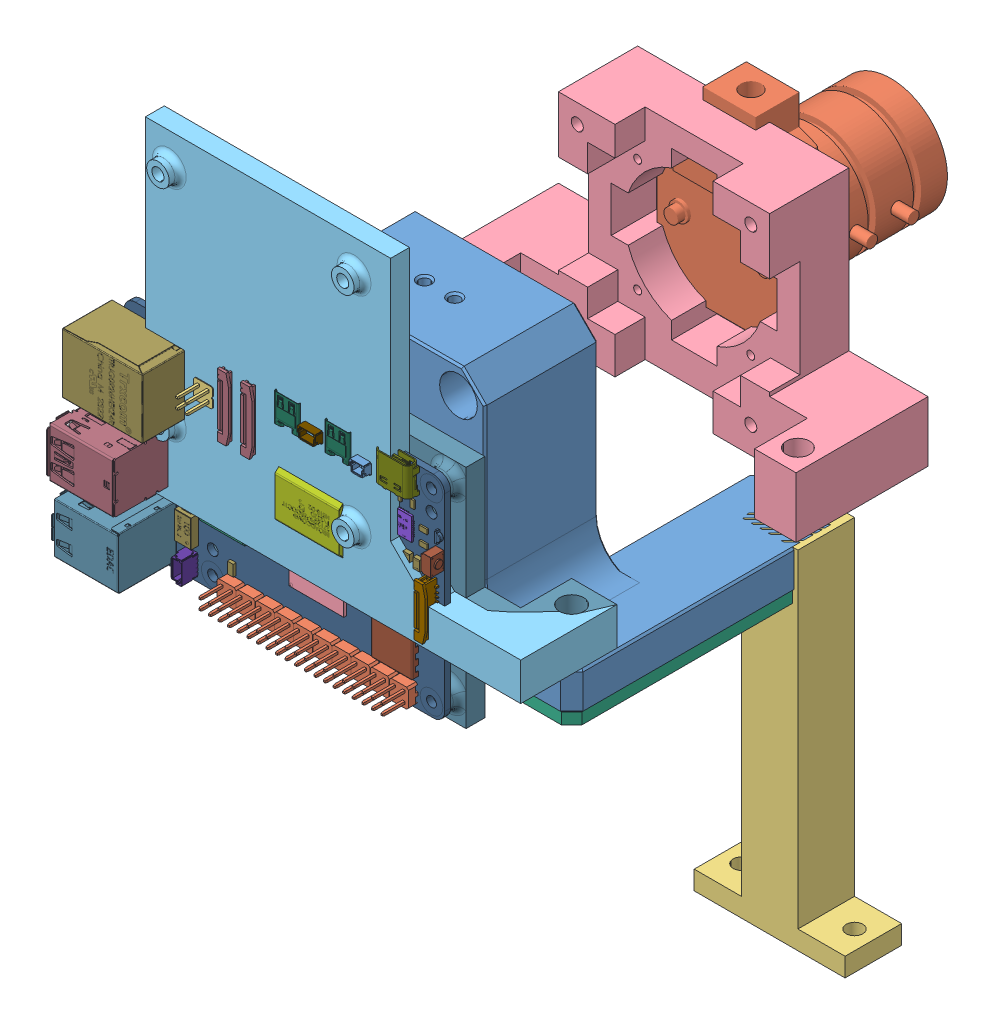
SolidWorks assembly Cam Existing setup, configuration Default. Lengths in mm.
Overall size (125.35 177 162.46).
37 component instances, 32 part files, 41 mates.
Components (placement in the parent):
- zaxismounting-1: zaxismounting [Default] at (-53.5245 -37.6157 41.3258) size (100 66.5 73)
- raspi_HQ_cam_and_6mm_lens-1: raspi_HQ_cam_and_6mm_lens [Default] at (-22.5245 33.3843 -47.4742) x (1 0 0) z (0 0 -1) size (38.99 51.7 46.02)
- Cam-Plate Spacer-1: Cam-Plate Spacer [Default] at (-3.5245 -27.6157 -51.1742) x (1 0 0) z (0 -1 0) size (40 15 92)
- Rpi Cam Mount 2-1: Rpi Cam Mount 2 [Default] at (-3.5245 2.3843 -41.1742) x (-1 0 0) z (0 0 -1) size (98 58 35)
- Rpi Mount-1: Rpi Mount [Default] at (-53.5245 -27.6157 41.3258) x (1 0 0) z (0 1 0) size (99.5 28.5 85)
- Spacer 3mm Zaxis mount^Cam Existing setup-1: Spacer 3mm Zaxis mount^Cam Existing setup [Default] at (-53.5245 -37.6157 41.3258) x (-1 0 0) z (0 -1 0) size (99 72 3)
- RASPBERRY_PI_5-2: RASPBERRY_PI_5 [Default] at (-18.9805 -16.8057 50.4258) x (-1 0 0) z (0 1 0) size (89.04 20.84 57.19)
  - RASPBERRY_PI_5.STEP-1: RASPBERRY_PI_5.STEP [Default] at origin size (89.04 20.84 57.19)
    - SLOT_CARD_ASM.STEP-1: SLOT_CARD_ASM.STEP [Default] at (-44.5448 -12.71 -6.4393) x (0 0 -1) z (0 1 0) size (11.95 11.4 1.48)
      - CARD_SLOT_METAL_PIN.STEP-1: CARD_SLOT_METAL_PIN.STEP [Default] at (-3.5293 -7.6678 12.2938) x (0 -1 0) z (1 0 0) size (7.95 0.89 8.04)
      - SD_CARD_V1.STEP-1: SD_CARD_V1.STEP [Default] at (-18.1743 -9.7848 12.71) x (-1 0 0) z (0 0 -1) size (11.71 10.28 1.3)
      - PART3_V1.STEP-1: PART3_V1.STEP [Default] at (-6.4643 -9.3448 11.38) x (1 0 0) z (0 0 -1) size (11.95 11.4 1.45)
    - PLATE_RASPBERRY_PI_5.STEP-1: PLATE_RASPBERRY_PI_5.STEP [Default] x (1 0 0) z (0 1 0) size (85 56 1.7)
    - METAL_PLATE..STEP-1: METAL_PLATE..STEP [Default] at (-30 3 -14.2) x (1 0 0) z (0 1 0) size (11.01 13.01 1.6)
    - GIGABIT_ETHERNET_PORT.STEP-1: GIGABIT_ETHERNET_PORT.STEP [Default] at (45.5 8.525 17.8) x (0 0 -1) z (1 0 0) size (16.1 17.2 21.45)
    - 2xUSB_3.0_PORT.STEP-1: 2xUSB_3.0_PORT.STEP [Default] at (28.53 10.58 -1.1) x (0 1 0) z (1 0 0) size (20.65 15.33 17.66)
    - 2xUSB_2.0_PORT.STEP-1: 2xUSB_2.0_PORT.STEP [Default] at (28.53 9.4 -19) x (0 1 0) z (1 0 0) size (19.16 15.33 17.86)
    - FEMALE_MICRO_HDMI_CONNECTOR.STEP-1: FEMALE_MICRO_HDMI_CONNECTOR.STEP [Default] at (-16.7 3.05 21.5) size (6.5 3.51 7.5)
    - FEMALE_MICRO_HDMI_CONNECTOR.STEP-2: FEMALE_MICRO_HDMI_CONNECTOR.STEP [Default] at (-3.3 3.05 21.5) size (6.5 3.51 7.5)
    - FEMALE_USB_CONNECTOR.STEP-1: FEMALE_USB_CONNECTOR.STEP [Default] at (-31.3 3.18 21.58) size (8.94 3.96 7.9)
    - STOCK_1.STEP-1: STOCK_1.STEP [Default] at (0.2694 -0.16 -24.2409) x (1 0 0) z (0 1 0) size (3.61 6 4.35)
    - STOCK_2.STEP-1: STOCK_2.STEP [Default] at (-10.7909 -0.16 48.1306) x (0 0 -1) z (0 1 0) size (3.61 5 4.35)
    - STOCK_3.STEP-1: STOCK_3.STEP [Default] at (-24.6409 -0.16 47.3806) x (0 0 -1) z (0 1 0) size (3.61 4 4.35)
    - 3.0_PIN_HEADER_10.STEP-1: 3.0_PIN_HEADER_10.STEP [Default] at (-32.86 4.1 -24.5) x (0 0 -1) z (0 1 0) size (5.08 50.8 11.8)
    - 2.0_PIN_HEADER.STEP-1: 2.0_PIN_HEADER.STEP [Default] at (19.04 4.1 18.56) x (1 0 0) z (0 1 0) size (5.08 5.08 11.8)
    - 9FD77_D9WHV.STEP-1: 9FD77_D9WHV.STEP [Default] at (-9.25 1.6 -11) x (0 0 1) z (0 1 0) size (10 14.5 0.8)
    - GIGABIT_ETHERNET_TRANSCEIVER.STEP-1: GIGABIT_ETHERNET_TRANSCEIVER.STEP [Default] at (21.5315 1.6 4.5573) x (0.707107 0 0.707107) z (0 1 0) size (6.9 6.9 1.1)
    - RP1_CO_CONTROLLER.STEP-1: RP1_CO_CONTROLLER.STEP [Default] at (15.9 1.6 -6.95) x (0 0 1) z (0 1 0) size (12 12 0.7)
    - BROADCOM_1.STEP-1: BROADCOM_1.STEP [Default] at (-0.825 4.78 5.305) x (0 0 1) z (-1 0 0) size (17 3.38 17)
    - MxL.STEP-1: MxL.STEP [Default] at (-31.24 1.6 12.88) x (0 0 1) z (0 1 0) size (6.48 6.48 0.6)
    - CAMERA_DISPLAY_1.STEP-1: CAMERA_DISPLAY_1.STEP [Default] at (-45.8516 -0.0005 -20.0821) x (1 0 0) z (0 1 0) size (3.5 13.7 3.9)
    - BUTTON_MINI.STEP-1: BUTTON_MINI.STEP [Default] at (0.19 4.2 29.7) x (1 0 0) z (0 -1 0) size (1.45 3.2 1)
    - BUTTON_2.STEP-1: BUTTON_2.STEP [Default] at (-41 1.6 9.6006) x (0 0 1) z (0 1 0) size (4.65 2.9 3.5)
    - CONNECT_V1.STEP-1: CONNECT_V1.STEP [Default] at (-5.5164 1.6 -0.8649) x (1 0 0) z (0 1 0) size (65.38 41.11 2)
    - CAMERA_DISPLAY_2.STEP-1: CAMERA_DISPLAY_2.STEP [Default] at (0.0484 -0.0005 -0.5921) x (1 0 0) z (0 1 0) size (3.5 16.7 3.9)
    - CAMERA_DISPLAY_2.STEP-2: CAMERA_DISPLAY_2.STEP [Default] at (6.2484 -0.0005 -0.5921) x (1 0 0) z (0 1 0) size (3.5 16.7 3.9)
- Rpi Mount2-1: Rpi Mount2 [Default] at (-53.5245 -27.6157 41.3258) x (1 0 0) z (0 1 0) size (99.5 21.5 60)
Mates (geometry in assembly coordinates):
- Concentric5: concentric anti-aligned: cylinder of zaxismounting-1 through (-47.0245 -37.6157 -25.1742) axis (0 -1 0) radius 3.5; cylinder of Rpi Cam Mount-1 through (-47.0245 -27.6157 -25.1742) axis (0 1 0) radius 3.1
- Concentric6: concentric anti-aligned: cylinder of zaxismounting-1 through (39.9755 -37.6157 -25.1742) axis (0 -1 0) radius 3.5; cylinder of Rpi Cam Mount-1 through (39.9755 -27.6157 -25.1742) axis (0 1 0) radius 3.1
- Concentric7: concentric aligned: cylinder of Rpi Cam Mount-1 through (-3.5245 2.3843 -38.1742) axis (0 0 -1) radius 18.5; line of raspi_HQ_cam_and_6mm_lens-1 through (-3.5245 2.3843 -63.1742) axis (0 0 -1)
- Coincident1: coincident anti-aligned: plane of Rpi Cam Mount-1 through (-3.5245 2.3843 -58.1742) normal (0 0 1); plane of raspi_HQ_cam_and_6mm_lens-1 through (-22.5245 33.3843 -63.1742) normal (0 0 -1)
- Parallel3: parallel anti-aligned: plane of Rpi Cam Mount-1 through (-3.5245 2.3843 -46.1742) normal (0 1 0); plane of raspi_HQ_cam_and_6mm_lens-1 through (-22.5245 33.3843 -47.4742) normal (0 -1 0)
- Coincident3: coincident anti-aligned: plane of zaxismounting-1 through (-53.5245 -27.6157 41.3258) normal (0 1 0); plane of Rpi Cam Mount-1 through (-3.5245 -27.6157 -46.1742) normal (0 -1 0)
- Concentric8: concentric anti-aligned: cylinder of zaxismounting-1 through (-47.0245 -37.6157 -25.1742) axis (0 -1 0) radius 3.5; cylinder of Rpi Cam Mount-2 through (-47.0245 -27.6157 -25.1742) axis (0 1 0) radius 3.1
- Concentric9: concentric anti-aligned: cylinder of zaxismounting-1 through (39.9755 -37.6157 -25.1742) axis (0 -1 0) radius 3.5; cylinder of Rpi Cam Mount-2 through (39.9755 -27.6157 -25.1742) axis (0 1 0) radius 3.1
- Concentric10: concentric anti-aligned: cylinder of zaxismounting-1 through (-47.0245 -37.6157 34.8258) axis (0 -1 0) radius 3.5; cylinder of Rpi Cam Mount-2 through (-47.0245 -27.6157 34.8258) axis (0 1 0) radius 3.1
- Coincident9: coincident anti-aligned: plane of zaxismounting-1 through (-53.5245 -27.6157 41.3258) normal (0 1 0); plane of Rpi Cam Mount-2 through (-3.5245 -27.6157 -51.1742) normal (0 -1 0)
- Coincident11: coincident: line of raspi_HQ_cam_and_6mm_lens-1 through (-3.5245 2.3843 -63.1742) axis (0 0 -1); plane of Rpi Cam Mount-2 through (-3.5245 2.3843 -51.1742) normal (0 1 0)
- Coincident12: coincident: line of raspi_HQ_cam_and_6mm_lens-1 through (-3.5245 2.3843 -63.1742) axis (0 0 -1); plane of Rpi Cam Mount-2 through (-3.5245 2.3843 -51.1742) normal (-1 0 0)
- Coincident14: coincident anti-aligned: plane of raspi_HQ_cam_and_6mm_lens-1 through (-22.5245 33.3843 -63.1742) normal (0 0 -1); plane of Rpi Cam Mount-2 through (-3.5245 2.3843 -63.1742) normal (0 0 1)
- InPlace1: in place: plane of ? through (-3.5245 -27.6157 -51.1742) normal (0 -1 0); plane of ? through (0 -27.6157 0) normal (0 -1 0); moOrthogonalPlaneRef_w of ? through (-3.5245 -27.6157 -51.1742) normal (0 -1 0); plane of ? through (0 -27.6157 0) normal (0 0 -1); plane of ? through (-3.5245 -27.6157 -51.1742) normal (0 -1 0); plane of ? through (0 -27.6157 0) normal (-1 0 0); plane of ? through (-3.5245 -27.6157 -51.1742) normal (0 -1 0); unknown of Cam-Plate Spacer-1
- Coincident15: coincident aligned: plane of ?; plane of Cam-Plate Spacer-1
- Coincident16: coincident aligned: moOrthogonalPlaneRef_w of Rpi Cam Mount-2 through (-3.5245 -27.6157 -51.1742) normal (0 0 1); plane of Cam-Plate Spacer-1 through (-3.5245 -27.6157 -51.1742) normal (0 0 1)
- Coincident17: coincident anti-aligned: moOrthogonalPlaneRef_w of Rpi Cam Mount-2 through (-3.5245 -27.6157 -51.1742) normal (-1 0 0); plane of Cam-Plate Spacer-1 through (-3.5245 -27.6157 -51.1742) normal (1 0 0)
- InPlace2: in place: plane of zaxismounting-1 through (-53.5245 -27.6157 41.3258) normal (0 1 0); plane of ? through (0 -27.6157 0) normal (0 1 0); plane of zaxismounting-1 through (-53.5245 -27.6157 41.3258) normal (0 1 0); plane of ? through (0 -27.6157 0) normal (0 0 -1); plane of zaxismounting-1 through (-53.5245 -27.6157 41.3258) normal (0 1 0); plane of ? through (0 -27.6157 0) normal (1 0 0); plane of zaxismounting-1 through (-53.5245 -27.6157 41.3258) normal (0 1 0); unknown of ?
- Coincident18: coincident aligned: plane of zaxismounting-1; plane of ?
- Coincident19: coincident aligned: moOrthogonalPlaneRef_w of zaxismounting-1 through (-53.5245 -27.6157 41.3258) normal (0 0 -1); plane of Part2^Cam Existing setup-1 through (-53.5245 -27.6157 41.3258) normal (0 0 -1)
- Coincident20: coincident anti-aligned: moOrthogonalPlaneRef_w of zaxismounting-1 through (-53.5245 -27.6157 41.3258) normal (-1 0 0); plane of Part2^Cam Existing setup-1 through (-53.5245 -27.6157 41.3258) normal (1 0 0)
- InPlace3: in place: plane of zaxismounting-1 through (-53.5245 -27.6157 41.3258) normal (0 1 0); plane of ? through (0 -27.6157 0) normal (0 1 0); plane of zaxismounting-1 through (-53.5245 -27.6157 41.3258) normal (0 1 0); plane of ? through (0 -27.6157 0) normal (0 0 -1); plane of zaxismounting-1 through (-53.5245 -27.6157 41.3258) normal (0 1 0); plane of ? through (0 -27.6157 0) normal (1 0 0); plane of zaxismounting-1 through (-53.5245 -27.6157 41.3258) normal (0 1 0); unknown of ?
- Coincident21: coincident aligned: plane of zaxismounting-1; plane of Rpi Mount-1
- Coincident22: coincident aligned: moOrthogonalPlaneRef_w of zaxismounting-1 through (-53.5245 -27.6157 41.3258) normal (0 0 -1); plane of Part3^Cam Existing setup-1 through (-53.5245 -27.6157 41.3258) normal (0 0 -1)
- Coincident23: coincident anti-aligned: moOrthogonalPlaneRef_w of zaxismounting-1 through (-53.5245 -27.6157 41.3258) normal (-1 0 0); plane of Part3^Cam Existing setup-1 through (-53.5245 -27.6157 41.3258) normal (1 0 0)
- InPlace4: in place: plane of zaxismounting-1 through (-53.5245 -37.6157 41.3258) normal (0 -1 0); plane of ? through (0 -37.6157 0) normal (0 -1 0); plane of zaxismounting-1 through (-53.5245 -37.6157 41.3258) normal (0 -1 0); plane of ? through (0 -37.6157 0) normal (0 0 -1); plane of zaxismounting-1 through (-53.5245 -37.6157 41.3258) normal (0 -1 0); plane of ? through (0 -37.6157 0) normal (-1 0 0); plane of zaxismounting-1 through (-53.5245 -37.6157 41.3258) normal (0 -1 0); unknown of Spacer 3mm Zaxis mount^Cam Existing setup-1
- Coincident15: coincident aligned: plane of zaxismounting-1; plane of Spacer 3mm Zaxis mount^Cam Existing setup-1
- Coincident16: coincident aligned: moOrthogonalPlaneRef_w of zaxismounting-1 through (-53.5245 -37.6157 41.3258) normal (0 0 -1); plane of Spacer 3mm Zaxis mount^Cam Existing setup-1 through (-53.5245 -37.6157 41.3258) normal (0 0 -1)
- Coincident17: coincident anti-aligned: moOrthogonalPlaneRef_w of zaxismounting-1 through (-53.5245 -37.6157 41.3258) normal (1 0 0); plane of Spacer 3mm Zaxis mount^Cam Existing setup-1 through (-53.5245 -37.6157 41.3258) normal (-1 0 0)
- Coincident18: coincident anti-aligned: plane of Rpi Cam Mount-2 through (-3.5245 2.3843 -51.1742) normal (-1 0 0); plane of RASPBERRY_PI_5-1 through (-3.5245 29.842 58.3258) normal (1 0 0)
- Distance1: distance = 4 mm anti-aligned: plane of RASPBERRY_PI_5-1/RASPBERRY_PI_5.STEP-1/PLATE_RASPBERRY_PI_5.STEP-1 through (2.2855 -9.658 58.3258) normal (0 0 -1); plane of Part3^Cam Existing setup-1 through (45.9755 -17.6157 54.3258) normal (0 0 1)
- Coincident20: coincident aligned: plane of Rpi Cam Mount-2 through (-3.5245 2.3843 -51.1742) normal (0 1 0); plane of RASPBERRY_PI_5-2 through (-18.9805 2.3843 50.4258) normal (0 1 0)
- Concentric12: concentric anti-aligned: cylinder of zaxismounting-1 through (39.9755 -37.6157 -25.1742) axis (0 -1 0) radius 3.5; cylinder of Rpi Cam Mount 2-1 through (39.9755 -27.6157 -25.1742) axis (0 1 0) radius 3.1
- Concentric13: concentric anti-aligned: cylinder of zaxismounting-1 through (-47.0245 -37.6157 -25.1742) axis (0 -1 0) radius 3.5; cylinder of Rpi Cam Mount 2-1 through (-47.0245 -27.6157 -25.1742) axis (0 1 0) radius 3.1
- Coincident21: coincident anti-aligned: plane of zaxismounting-1 through (-53.5245 -27.6157 41.3258) normal (0 1 0); plane of Rpi Cam Mount 2-1 through (-3.5245 -27.6157 -41.1742) normal (0 -1 0)
- Concentric14: concentric aligned: cylinder of zaxismounting-1 through (39.9755 -37.6157 34.8258) axis (0 -1 0) radius 3.5; cylinder of Rpi Mount2-1 through (39.9755 -17.6157 34.8258) axis (0 -1 0) radius 3.2
- Coincident22: coincident anti-aligned: plane of zaxismounting-1 through (-53.5245 -27.6157 41.3258) normal (0 1 0); plane of Rpi Mount2-1 through (-53.5245 -27.6157 41.3258) normal (0 -1 0)
- Concentric15: concentric aligned: cylinder of zaxismounting-1 through (-47.0245 -37.6157 34.8258) axis (0 -1 0) radius 3.5; cylinder of Rpi Mount2-1 through (-47.0245 -17.6157 34.8258) axis (0 -1 0) radius 3.2
- Coincident23: coincident anti-aligned: plane of Rpi Cam Mount 2-1 through (-3.5245 2.3843 -41.1742) normal (0 1 0); plane of RASPBERRY_PI_5-3 through (8.4362 2.3843 50.3258) normal (0 -1 0)
- Coincident24: coincident anti-aligned: plane of Rpi Mount2-1 through (20.0195 7.6943 50.3258) normal (0 0 1); plane of RASPBERRY_PI_5-3/RASPBERRY_PI_5.STEP-1/PLATE_RASPBERRY_PI_5.STEP-1 through (-31.0638 -3.4257 50.3258) normal (0 0 -1)
- Coincident25: coincident anti-aligned: plane of RASPBERRY_PI_5-2/RASPBERRY_PI_5.STEP-1/PLATE_RASPBERRY_PI_5.STEP-1 through (-37.9805 -41.3057 50.3258) normal (0 0 -1); plane of Rpi Mount2-1 through (-37.9805 -41.3057 50.3258) normal (0 0 1)
